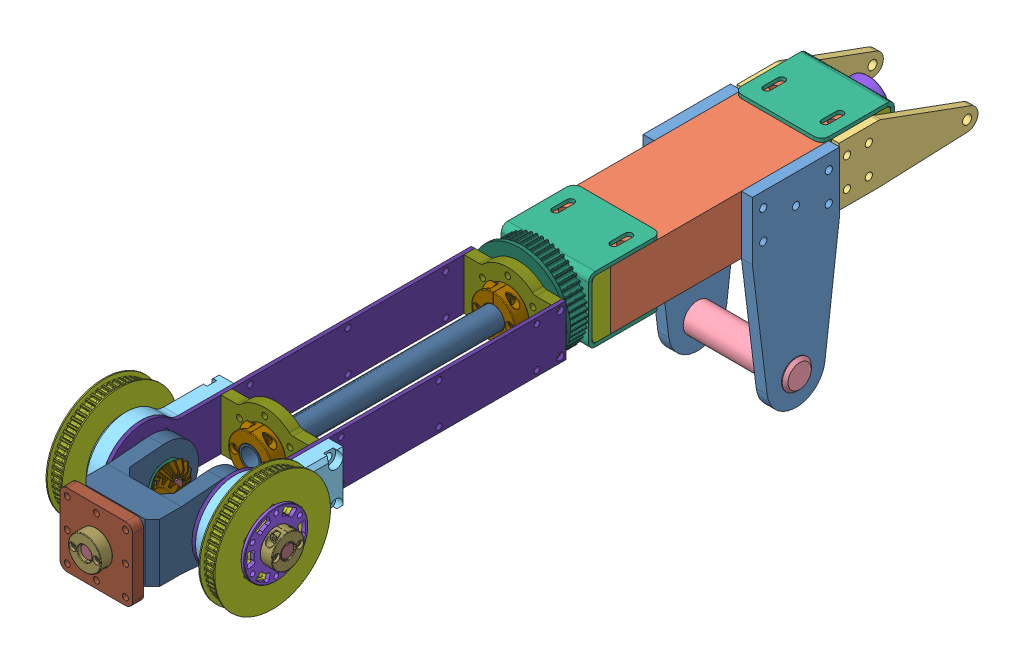
SolidWorks assembly Forearm, configuration Default. Lengths in mm.
Overall size (174.26 202.9 760.46).
74 component instances, 31 part files, 63 mates.
Components (placement in the parent):
- SidePlate^Forearm-1: SidePlate^Forearm [Default] at origin size (9.52 177.8 76.2) (virtual)
- SidePlate^Forearm-2: SidePlate^Forearm [Default] x (-1 0 0) z (0 0 -1) size (9.52 177.8 76.2) (virtual)
- Box^Forearm-1: Box^Forearm [Default] at origin size (76.2 50.8 228.6) (virtual)
- BackSidePlate^Forearm-1: BackSidePlate^Forearm [Default] at origin size (6.35 73.03 146.68) (virtual)
- BackSidePlate^Forearm-2: BackSidePlate^Forearm [Default] at (82.55 0 0) size (6.35 73.03 146.68) (virtual)
- 6061K602_HARDENED PRECISION STEEL SHAFT-1: 6061K602_HARDENED PRECISION STEEL SHAFT [6061K602] at (0 609.075 0) size (101.6 25.4 25.4)
- 6384K367_BALL BEARING-1: 6384K367_BALL BEARING [6384K367] at (0 736.075 166.624) x (1 0 0) z (0 0 -1) size (44.45 44.45 14.3)
- BearingHolder^Forearm-1: BearingHolder^Forearm [Default] at origin size (76.2 57.15 63.5) (virtual)
- BearingSpacer^Forearm-1: BearingSpacer^Forearm [Default] at origin size (76.2 50.8 22.22) (virtual)
- BearingSpacer^Forearm-2: BearingSpacer^Forearm [Default] at (0 0 76.2) x (-1 0 0) z (0 0 -1) size (76.2 50.8 22.22) (virtual)
- BearingHolder^Forearm-2: BearingHolder^Forearm [Default] at (0 0 76.2) x (-1 0 0) z (0 0 -1) size (76.2 57.15 63.5) (virtual)
- 6384K367_BALL BEARING-2: 6384K367_BALL BEARING [6384K367] at (0 736.075 -90.424) x (-1 0 0) z (0 0 1) size (44.45 44.45 14.3)
- 6435K160_ONE-PIECE CLAMP-ON SHAFT COLLAR-1: 6435K160_ONE-PIECE CLAMP-ON SHAFT COLLAR [6435K16] at (0 736.075 -104.7242) x (1 0 0) z (0 0 -1) size (38.1 38.11 12.77)
- 9677T100_CLAMP-ON SHAFT COLLAR WITH MOUNTING HOLES-1: 9677T100_CLAMP-ON SHAFT COLLAR WITH MOUNTING HOLES [9677T1] at (0 736.075 210.2517) x (0 -1 0) z (0 0 -1) size (38.14 38.1 13.27)
- 89955K599_Tube^Forearm-1: 89955K599_Tube^Forearm [Default] at origin size (19.05 19.05 539.7) (virtual)
- ThrustBase^Forearm-1: ThrustBase^Forearm [Default] at origin size (44.45 44.45 8.27) (virtual)
- 5909K460_THRUST NEEDLE-ROLLER BEARING-1: 5909K460_THRUST NEEDLE-ROLLER BEARING [5909K46] at (0 736.075 182.0545) x (0 0 -1) z (1 0 0) size (0.81 31.75 31.75)
- 5909K330_THRUST NEEDLE-ROLLER BEARING-1: 5909K330_THRUST NEEDLE-ROLLER BEARING [5909K33] at (0 736.075 183.0467) x (1 0 0) z (0 1 0) size (31.75 1.98 31.75)
- 5909K460_THRUST NEEDLE-ROLLER BEARING-2: 5909K460_THRUST NEEDLE-ROLLER BEARING [5909K46] at (0 736.075 184.8517) x (0 0 -1) z (1 0 0) size (0.81 31.75 31.75)
- PulleySupportPlate^Forearm-1: PulleySupportPlate^Forearm [Default] at origin size (63.5 63.5 3.18) (virtual)
- J4Pulley-1: J4Pulley [Default] at (0 736.075 191.2017) x (-1 0 0) z (0 -1 0) size (84.06 20.68 84.06)
- WristHub^Forearm-1: WristHub^Forearm [Default] at origin size (76.2 63.5 9.53) (virtual)
- WristSidePlate^Forearm-1: WristSidePlate^Forearm [Default] at origin size (3.17 69.85 323.15) (virtual)
- WristSidePlate^Forearm-2: WristSidePlate^Forearm [Default] at (79.375 0 0) size (3.17 69.85 323.15) (virtual)
- WristHub^Forearm-2: WristHub^Forearm [Default] at (0 0 212.0233) size (76.2 63.5 9.53) (virtual)
- 9677T100_CLAMP-ON SHAFT COLLAR WITH MOUNTING HOLES-2: 9677T100_CLAMP-ON SHAFT COLLAR WITH MOUNTING HOLES [9677T1] at (0 736.075 422.275) x (0 -1 0) z (0 0 -1) size (38.14 38.1 13.27)
- 6843K130_MTL MITER GEAR--20 DEG PRESSURE ANGLE-1: 6843K130_MTL MITER GEAR--20 DEG PRESSURE ANGLE [6843K13] at (-31.1638 691.933 470.788) x (0 -0.999847 0.017483) z (0 0.017483 0.999847) size (34.68 21.82 34.5)
- 6843K130_MTL MITER GEAR--20 DEG PRESSURE ANGLE-3: 6843K130_MTL MITER GEAR--20 DEG PRESSURE ANGLE [6843K13] at (-11.812 691.933 513.7638) x (0.017483 -0.999847 0) z (0.999847 0.017483 0) size (34.68 21.82 34.5)
- 6384K361_BALL BEARING-1-1: 6384K361_BALL BEARING-1 [6384K361] at (-41.3385 736.075 482.6) x (0 0 1) z (-1 0 0) size (31.75 31.75 11.13)
- 5909K440_THRUST NEEDLE-ROLLER BEARING-1: 5909K440_THRUST NEEDLE-ROLLER BEARING [5909K44] at (-34.5472 736.075 482.6) size (0.81 23.81 23.81)
- 5909K310_THRUST NEEDLE-ROLLER BEARING-1: 5909K310_THRUST NEEDLE-ROLLER BEARING [5909K31] at (-32.7422 736.075 482.6) x (0 1 0) z (0 0 1) size (23.81 1.98 23.81)
- MiterSpacer^Forearm-1: MiterSpacer^Forearm [Default] at origin size (2.03 31.75 31.75) (virtual)
- SidePrintedSupport^Forearm-1: SidePrintedSupport^Forearm [Default] at origin size (15.88 69.85 115.89) (virtual)
- 6384K361_BALL BEARING-1-2: 6384K361_BALL BEARING-1 [6384K361] at (-53.9115 736.075 482.6) x (0 0 1) z (1 0 0) size (31.75 31.75 11.13)
- SidePrintedSupport^Forearm-2: SidePrintedSupport^Forearm [Default] at (0 1472.15 0) x (-1 0 0) z (0 0 1) size (15.88 69.85 115.89) (virtual)
- 6384K361_BALL BEARING-1-3: 6384K361_BALL BEARING-1 [6384K361] at (53.9115 736.075 482.6) x (0 0 -1) z (-1 0 0) size (31.75 31.75 11.13)
- 6384K361_BALL BEARING-1-4: 6384K361_BALL BEARING-1 [6384K361] at (41.3385 736.075 482.6) x (0 0 -1) z (1 0 0) size (31.75 31.75 11.13)
- MiterSpacer^Forearm-2: MiterSpacer^Forearm [Default] at (0 0 965.2) x (-1 0 0) z (0 0 -1) size (2.03 31.75 31.75) (virtual)
- 5909K440_THRUST NEEDLE-ROLLER BEARING-2: 5909K440_THRUST NEEDLE-ROLLER BEARING [5909K44] at (34.5472 736.075 482.6) x (-1 0 0) z (0 0 -1) size (0.81 23.81 23.81)
- 5909K310_THRUST NEEDLE-ROLLER BEARING-2: 5909K310_THRUST NEEDLE-ROLLER BEARING [5909K31] at (32.7422 736.075 482.6) x (0 1 0) z (0 0 1) size (23.81 1.98 23.81)
- 6843K130_MTL MITER GEAR--20 DEG PRESSURE ANGLE-4: 6843K130_MTL MITER GEAR--20 DEG PRESSURE ANGLE [6843K13] at (31.1638 779.7771 469.252) x (0 0.999847 -0.017483) z (0 0.017483 0.999847) size (34.68 21.82 34.5)
- 6391K281_OIL-EMBEDDED SLEEVE BEARING-1: 6391K281_OIL-EMBEDDED SLEEVE BEARING [6391K281] at (-25.8945 736.075 482.6) x (0 0 1) z (-1 0 0) size (31.78 31.78 12.7)
- 6391K281_OIL-EMBEDDED SLEEVE BEARING-2: 6391K281_OIL-EMBEDDED SLEEVE BEARING [6391K281] at (25.8945 736.075 482.6) x (0 0 1) z (-1 0 0) size (31.78 31.78 12.7)
- PulleyHubbed-1: PulleyHubbed [Default] at (-79.0217 736.075 482.6) x (0 0 1) z (-1 0 0) size (101 101 17.18)
  - 60t_x_18mm_Wide_VersaPulley_Kit_HTD_5mm_VersaKeys_217-3200 v2-1: 60t_x_18mm_Wide_VersaPulley_Kit_HTD_5mm_VersaKeys_217-3200 v2 [Default] at origin size (101 101 14)
    - 60t_x_18mm_Wide_VersaPulley_Kit_HTD_5mm_VersaKeys_217-3200 v2.step-1: 60t_x_18mm_Wide_VersaPulley_Kit_HTD_5mm_VersaKeys_217-3200 v2.step [Default] at origin size (101 101 14)
      - 217-3200-001 Rev3.step-1: 217-3200-001 Rev3.step [Default] at (0 0 -7) size (101 101 10.18)
      - 217-3200-001 Rev3.step-2: 217-3200-001 Rev3.step [Default] at (0 0 -17.825) x (-1 0 0) z (0 0 -1) size (101 101 10.18)
  - 1_2_ID_1_8_Keyway_Aluminum_VersaHub_217-2590 v1-1: 1_2_ID_1_8_Keyway_Aluminum_VersaHub_217-2590 v1 [Default] at (0 0 -14.9375) x (0 0 1) z (1 0 0) size (12.7 55.88 55.88)
- SidePulleySpacer^Forearm-1: SidePulleySpacer^Forearm [Default] at origin size (3.81 17.78 17.78) (virtual)
- PulleyHubbed-2: PulleyHubbed [Default] at (79.0217 736.075 482.6) x (0 0 -1) z (1 0 0) size (101 101 17.18)
  - 60t_x_18mm_Wide_VersaPulley_Kit_HTD_5mm_VersaKeys_217-3200 v2-1: 60t_x_18mm_Wide_VersaPulley_Kit_HTD_5mm_VersaKeys_217-3200 v2 [Default] at origin size (101 101 14)
    - 60t_x_18mm_Wide_VersaPulley_Kit_HTD_5mm_VersaKeys_217-3200 v2.step-1: 60t_x_18mm_Wide_VersaPulley_Kit_HTD_5mm_VersaKeys_217-3200 v2.step [Default] at origin size (101 101 14)
      - 217-3200-001 Rev3.step-1: 217-3200-001 Rev3.step [Default] at (0 0 -7) size (101 101 10.18)
      - 217-3200-001 Rev3.step-2: 217-3200-001 Rev3.step [Default] at (0 0 -17.825) x (-1 0 0) z (0 0 -1) size (101 101 10.18)
  - 1_2_ID_1_8_Keyway_Aluminum_VersaHub_217-2590 v1-1: 1_2_ID_1_8_Keyway_Aluminum_VersaHub_217-2590 v1 [Default] at (0 0 -14.9375) x (0 0 1) z (1 0 0) size (12.7 55.88 55.88)
- SidePulleySpacer^Forearm-2: SidePulleySpacer^Forearm [Default] at (0 0 965.2) x (-1 0 0) z (0 0 -1) size (3.81 17.78 17.78) (virtual)
- WristBase^Forearm-3: WristBase^Forearm [Default] at origin size (64.49 57.15 92.08) (virtual)
- 6384K361_BALL BEARING-1-5: 6384K361_BALL BEARING-1 [6384K361] at (0 736.075 523.9385) size (31.75 31.75 11.13)
- MiterSpacer^Forearm-3: MiterSpacer^Forearm [Default] at (-482.6 0 482.6) x (0 0 -1) z (1 0 0) size (2.03 31.75 31.75) (virtual)
- 5909K440_THRUST NEEDLE-ROLLER BEARING-3: 5909K440_THRUST NEEDLE-ROLLER BEARING [5909K44] at (0 736.075 517.1472) x (0 0 -1) z (1 0 0) size (0.81 23.81 23.81)
- 5909K310_THRUST NEEDLE-ROLLER BEARING-3: 5909K310_THRUST NEEDLE-ROLLER BEARING [5909K31] at (0 736.075 515.3422) x (0 1 0) z (-1 0 0) size (23.81 1.98 23.81)
- 6384K361_BALL BEARING-1-6: 6384K361_BALL BEARING-1 [6384K361] at (0 736.075 542.8615) x (1 0 0) z (0 0 -1) size (31.75 31.75 11.13)
- MiterSpacer^Forearm-4: MiterSpacer^Forearm [Default] at (-482.6 0 513.0768) x (0 0 -1) z (1 0 0) size (2.03 31.75 31.75) (virtual)
- 5909K440_THRUST NEEDLE-ROLLER BEARING-4: 5909K440_THRUST NEEDLE-ROLLER BEARING [5909K44] at (0 736.075 550.4656) x (0 0 -1) z (1 0 0) size (0.81 23.81 23.81)
- 5909K440_THRUST NEEDLE-ROLLER BEARING-5: 5909K440_THRUST NEEDLE-ROLLER BEARING [5909K44] at (0 736.075 553.2628) x (0 0 -1) z (1 0 0) size (0.81 23.81 23.81)
- 5909K310_THRUST NEEDLE-ROLLER BEARING-4: 5909K310_THRUST NEEDLE-ROLLER BEARING [5909K31] at (0 736.075 551.4578) x (0 1 0) z (-1 0 0) size (23.81 1.98 23.81)
- HandPlate^Forearm-1: HandPlate^Forearm [Default] at origin size (63.5 63.5 9.52) (virtual)
- 9677T210_CLAMP-ON SHAFT COLLAR WITH MOUNTING HOLES-1: 9677T210_CLAMP-ON SHAFT COLLAR WITH MOUNTING HOLES [9677T21] at (0 736.075 567.9472) x (0 1 0) z (0 0 -1) size (28.6 28.57 10.69)
- 9677T210_CLAMP-ON SHAFT COLLAR WITH MOUNTING HOLES-2: 9677T210_CLAMP-ON SHAFT COLLAR WITH MOUNTING HOLES [9677T21] at (-81.9436 736.075 482.6) x (0 -1 0) z (1 0 0) size (28.6 28.57 10.69)
- 9677T210_CLAMP-ON SHAFT COLLAR WITH MOUNTING HOLES-3: 9677T210_CLAMP-ON SHAFT COLLAR WITH MOUNTING HOLES [9677T21] at (81.9436 736.075 482.6) x (0 -1 0) z (-1 0 0) size (28.6 28.57 10.69)
- 8488T310_FULLY KEYED PRECISION DRIVE SHAFT W CERT-1: 8488T310_FULLY KEYED PRECISION DRIVE SHAFT W CERT [8488T31] at (-48.5172 736.075 482.6) x (0 0 1) z (-1 0 0) size (12.7 12.5 76.2)
- 8488T310_FULLY KEYED PRECISION DRIVE SHAFT W CERT-2: 8488T310_FULLY KEYED PRECISION DRIVE SHAFT W CERT [8488T31] at (48.5172 736.075 482.6) x (0 0 1) z (-1 0 0) size (12.7 12.5 76.2)
- 8488T310_FULLY KEYED PRECISION DRIVE SHAFT W CERT-3: 8488T310_FULLY KEYED PRECISION DRIVE SHAFT W CERT [8488T31] at (0 736.075 532.819) size (12.7 12.5 76.2)
Mates (geometry in assembly coordinates):
- Concentric1: concentric anti-aligned: cylinder of SidePlate^Forearm-1 through (-47.625 609.075 0) axis (1 0 0) radius 12.7; circle of 6061K602_HARDENED PRECISION STEEL SHAFT-1
- Width1: width anti-aligned: plane of 6061K602_HARDENED PRECISION STEEL SHAFT-1 through (-50.8 609.075 0) normal (-1 0 0); plane of SidePlate^Forearm-2 through (50.8 609.075 0) normal (1 0 0); plane of 6061K602_HARDENED PRECISION STEEL SHAFT-1 through (47.625 609.075 0) normal (1 0 0); plane of SidePlate^Forearm-1 through (-47.625 609.075 0) normal (-1 0 0)
- Concentric2: concentric aligned: cylinder of 6384K367_BALL BEARING-1 through (0 736.075 160.274) axis (0 0 -1) radius 20.6375; cylinder of BearingHolder^Forearm-1 through (0 736.075 171.45) axis (0 0 -1) radius 20.6375
- Coincident2: coincident anti-aligned: plane of 6384K367_BALL BEARING-1 through (0 720.6646 171.45) normal (0 0 -1); plane of BearingHolder^Forearm-1 through (0 0 171.45) normal (0 0 1)
- Concentric3: concentric aligned: cylinder of 6384K367_BALL BEARING-2 through (0 736.075 -84.074) axis (0 0 1) radius 9.525; cylinder of 6435K160_ONE-PIECE CLAMP-ON SHAFT COLLAR-1 through (0 736.075 -111.0742) axis (0 0 1) radius 9.525
- Coincident3: coincident anti-aligned: plane of 6384K367_BALL BEARING-2 through (0 725.2038 -98.3742) normal (0 0 -1); plane of 6435K160_ONE-PIECE CLAMP-ON SHAFT COLLAR-1 through (0 736.075 -98.3742) normal (0 0 1)
- Concentric4: concentric anti-aligned: cylinder of 6384K367_BALL BEARING-1 through (0 736.075 160.274) axis (0 0 -1) radius 9.525; cylinder of 9677T100_CLAMP-ON SHAFT COLLAR WITH MOUNTING HOLES-1 through (0 736.075 203.9017) axis (0 0 1) radius 9.525
- Concentric5: concentric anti-aligned: cylinder of 89955K599_Tube^Forearm-1 through (0 736.075 455.5658) axis (0 0 -1) radius 9.525; cylinder of 5909K460_THRUST NEEDLE-ROLLER BEARING-1 through (0 736.075 181.2417) axis (0 0 1) radius 9.5504
- Coincident4: coincident anti-aligned: plane of ThrustBase^Forearm-1 through (0 736.075 181.2417) normal (0 0 1); plane of 5909K460_THRUST NEEDLE-ROLLER BEARING-1 through (0 736.075 181.2417) normal (0 0 -1)
- Concentric6: concentric anti-aligned: cylinder of 89955K599_Tube^Forearm-1 through (0 736.075 455.5658) axis (0 0 -1) radius 9.525; cylinder of 5909K330_THRUST NEEDLE-ROLLER BEARING-1 through (0 736.075 184.0389) axis (0 0 1) radius 9.5504
- Tangent1: tangent anti-aligned: plane of 5909K460_THRUST NEEDLE-ROLLER BEARING-1 through (0 736.075 182.0545) normal (0 0 1); cylinder of 5909K330_THRUST NEEDLE-ROLLER BEARING-1 through (-5.4469 722.3178 183.0467) axis (-0.368125 -0.929776 0) radius 0.9922
- Concentric7: concentric anti-aligned: cylinder of 89955K599_Tube^Forearm-1 through (0 736.075 455.5658) axis (0 0 -1) radius 9.525; cylinder of 5909K460_THRUST NEEDLE-ROLLER BEARING-2 through (0 736.075 184.0389) axis (0 0 1) radius 9.5504
- Tangent2: tangent anti-aligned: cylinder of 5909K330_THRUST NEEDLE-ROLLER BEARING-1 through (-1.8545 721.3954 183.0467) axis (-0.125333 -0.992115 0) radius 0.9922; plane of 5909K460_THRUST NEEDLE-ROLLER BEARING-2 through (0 736.075 184.0389) normal (0 0 -1)
- Concentric8: concentric anti-aligned: cylinder of 89955K599_Tube^Forearm-1 through (0 736.075 455.5658) axis (0 0 -1) radius 9.525; circle of J4Pulley-1
- Coincident6: coincident anti-aligned: plane of PulleySupportPlate^Forearm-1 through (0 0 188.0267) normal (0 0 1); plane of J4Pulley-1 through (0 736.075 188.0267) normal (0 0 -1)
- Parallel1: parallel anti-aligned: plane of 9677T100_CLAMP-ON SHAFT COLLAR WITH MOUNTING HOLES-1 through (0.0953 755.1248 203.9017) normal (-1 0 0)
- Coincident11: coincident anti-aligned: plane of 9677T100_CLAMP-ON SHAFT COLLAR WITH MOUNTING HOLES-1 through (0 736.075 203.9017) normal (0 0 -1); plane of WristBase^Forearm-1 through (-24.5934 763.0625 203.9017) normal (0 0 1)
- Concentric10: concentric aligned: cylinder of 89955K599_Tube^Forearm-1 through (0 736.075 455.5658) axis (0 0 -1) radius 9.525; cylinder of WristHub^Forearm-2 through (0 736.075 415.925) axis (0 0 -1) radius 9.525
- Distance2: distance = 406.4 mm: plane of assembly through (0 0 0) normal (0 0 1); plane of WristBase^Forearm-2 through (-24.5934 763.0625 406.4) normal (0 0 -1)
- Concentric11: concentric anti-aligned: cylinder of 89955K599_Tube^Forearm-1 through (0 736.075 455.5658) axis (0 0 -1) radius 7.9375; cylinder of 9677T100_CLAMP-ON SHAFT COLLAR WITH MOUNTING HOLES-2 through (0 736.075 415.925) axis (0 0 1) radius 9.525
- Coincident13: coincident anti-aligned: plane of WristHub^Forearm-2 through (-24.5934 763.0625 415.925) normal (0 0 1); plane of 9677T100_CLAMP-ON SHAFT COLLAR WITH MOUNTING HOLES-2 through (0 736.075 415.925) normal (0 0 -1)
- Concentric12: concentric anti-aligned: cylinder of WristSidePlate^Forearm-1 through (-41.275 736.075 482.6) axis (1 0 0) radius 14.2875; cylinder of 6843K130_MTL MITER GEAR--20 DEG PRESSURE ANGLE-1 through (31.0355 736.075 482.6) axis (-1 0 0) radius 6.3563
- Concentric13: concentric anti-aligned: cylinder of 89955K599_Tube^Forearm-1 through (0 736.075 455.5658) axis (0 0 -1) radius 7.9375; cylinder of 6843K130_MTL MITER GEAR--20 DEG PRESSURE ANGLE-3 through (0 736.075 451.5645) axis (0 0 1) radius 6.3563
- Distance3: distance = 31.75 mm: cylinder of 6843K130_MTL MITER GEAR--20 DEG PRESSURE ANGLE-3 through (0 736.075 451.5645) axis (0 0 1) radius 6.3563; plane of 6843K130_MTL MITER GEAR--20 DEG PRESSURE ANGLE-1 through (-31.75 735.853 469.9019) normal (-1 0 0)
- Distance4: distance = 31.75 mm: plane of 6843K130_MTL MITER GEAR--20 DEG PRESSURE ANGLE-3 through (-12.6981 735.853 514.35) normal (0 0 1); cylinder of 6843K130_MTL MITER GEAR--20 DEG PRESSURE ANGLE-1 through (31.0355 736.075 482.6) axis (-1 0 0) radius 6.3563
- Concentric14: concentric anti-aligned: cylinder of WristSidePlate^Forearm-1 through (-41.275 736.075 482.6) axis (1 0 0) radius 14.2875; cylinder of 6384K361_BALL BEARING-1-1 through (-46.101 736.075 482.6) axis (-1 0 0) radius 14.2875
- Coincident14: coincident anti-aligned: plane of WristSidePlate^Forearm-1 through (-38.1 701.15 450.2212) normal (1 0 0); plane of 6384K361_BALL BEARING-1-1 through (-38.1 746.7938 482.6) normal (-1 0 0)
- Concentric15: concentric aligned: cylinder of 6843K130_MTL MITER GEAR--20 DEG PRESSURE ANGLE-1 through (31.0355 736.075 482.6) axis (-1 0 0) radius 6.3563; cylinder of 5909K440_THRUST NEEDLE-ROLLER BEARING-1 through (-33.7344 736.075 482.6) axis (-1 0 0) radius 6.3754
- Concentric16: concentric anti-aligned: cylinder of 6843K130_MTL MITER GEAR--20 DEG PRESSURE ANGLE-1 through (31.0355 736.075 482.6) axis (-1 0 0) radius 6.3563; cylinder of 5909K310_THRUST NEEDLE-ROLLER BEARING-1 through (-31.75 736.075 482.6) axis (1 0 0) radius 6.3754
- Tangent6: tangent anti-aligned: plane of 6843K130_MTL MITER GEAR--20 DEG PRESSURE ANGLE-1 through (-31.75 735.853 469.9019) normal (-1 0 0); cylinder of 5909K310_THRUST NEEDLE-ROLLER BEARING-1 through (-32.7422 725.194 485.3554) axis (0 -0.9694 0.245485) radius 0.9922
- Tangent7: tangent anti-aligned: plane of 5909K440_THRUST NEEDLE-ROLLER BEARING-1 through (-33.7344 736.075 482.6) normal (1 0 0); cylinder of 5909K310_THRUST NEEDLE-ROLLER BEARING-1 through (-32.7422 725.194 485.3554) axis (0 -0.9694 0.245485) radius 0.9922
- Concentric17: concentric aligned: cylinder of SidePrintedSupport^Forearm-1 through (-57.15 736.075 482.6) axis (1 0 0) radius 14.2875; cylinder of 6384K361_BALL BEARING-1-2 through (-49.149 736.075 482.6) axis (1 0 0) radius 14.2875
- Coincident16: coincident anti-aligned: plane of SidePrintedSupport^Forearm-1 through (-57.15 0 0) normal (-1 0 0); plane of 6384K361_BALL BEARING-1-2 through (-57.15 725.3562 482.6) normal (1 0 0)
- Concentric18: concentric anti-aligned: cylinder of 6843K130_MTL MITER GEAR--20 DEG PRESSURE ANGLE-1 through (31.0355 736.075 482.6) axis (-1 0 0) radius 12.7; cylinder of 6391K281_OIL-EMBEDDED SLEEVE BEARING-1 through (-32.2445 736.075 482.6) axis (1 0 0) radius 12.7
- Concentric20: concentric anti-aligned: cylinder of 6384K361_BALL BEARING-1-2 through (-49.149 736.075 482.6) axis (1 0 0) radius 6.35; cylinder of PulleyHubbed-1/1_2_ID_1_8_Keyway_Aluminum_VersaHub_217-2590 v1-1 through (-64.0842 736.075 482.6) axis (-1 0 0) radius 6.3627
- Coincident18: coincident anti-aligned: plane of PulleyHubbed-1/1_2_ID_1_8_Keyway_Aluminum_VersaHub_217-2590 v1-1 through (-64.0842 736.075 482.6) normal (1 0 0); plane of SidePulleySpacer^Forearm-1 through (-64.0842 736.075 482.6) normal (-1 0 0)
- Concentric21: concentric anti-aligned: cylinder of WristBase^Forearm-3 through (0 736.075 546.1) axis (0 0 -1) radius 14.2875; cylinder of 6384K361_BALL BEARING-1-5 through (0 736.075 528.701) axis (0 0 1) radius 14.2875
- Coincident19: coincident anti-aligned: plane of WristBase^Forearm-3 through (0 0 520.7) normal (0 0 -1); plane of 6384K361_BALL BEARING-1-5 through (0 746.7938 520.7) normal (0 0 1)
- Concentric22: concentric anti-aligned: cylinder of WristBase^Forearm-3 through (0 736.075 546.1) axis (0 0 -1) radius 14.2875; cylinder of MiterSpacer^Forearm-3 through (0 736.075 472.2459) axis (0 0 1) radius 9.3726
- Coincident21: coincident anti-aligned: plane of 6384K361_BALL BEARING-1-5 through (0 749.8863 519.176) normal (0 0 -1); plane of MiterSpacer^Forearm-3 through (0 736.075 519.176) normal (0 0 1)
- Concentric23: concentric anti-aligned: cylinder of WristBase^Forearm-3 through (0 736.075 546.1) axis (0 0 -1) radius 14.2875; cylinder of 5909K440_THRUST NEEDLE-ROLLER BEARING-3 through (0 736.075 516.3344) axis (0 0 1) radius 6.3754
- Coincident22: coincident anti-aligned: plane of MiterSpacer^Forearm-3 through (0 736.075 517.1472) normal (0 0 -1); plane of 5909K440_THRUST NEEDLE-ROLLER BEARING-3 through (0 736.075 517.1472) normal (0 0 1)
- Concentric24: concentric anti-aligned: cylinder of WristBase^Forearm-3 through (0 736.075 546.1) axis (0 0 -1) radius 14.2875; cylinder of 5909K310_THRUST NEEDLE-ROLLER BEARING-3 through (0 736.075 516.3344) axis (0 0 1) radius 6.3754
- Tangent8: tangent anti-aligned: plane of 6843K130_MTL MITER GEAR--20 DEG PRESSURE ANGLE-3 through (-12.6981 735.853 514.35) normal (0 0 1); cylinder of 5909K310_THRUST NEEDLE-ROLLER BEARING-3 through (-8.8576 742.9692 515.3422) axis (-0.789141 0.614213 0) radius 0.9922
- Concentric25: concentric aligned: cylinder of WristBase^Forearm-3 through (0 736.075 546.1) axis (0 0 -1) radius 14.2875; cylinder of 6384K361_BALL BEARING-1-6 through (0 736.075 538.099) axis (0 0 -1) radius 14.2875
- Coincident24: coincident anti-aligned: plane of WristBase^Forearm-3 through (0 0 546.1) normal (0 0 1); plane of 6384K361_BALL BEARING-1-6 through (0 725.3562 546.1) normal (0 0 -1)
- Concentric26: concentric anti-aligned: cylinder of 6384K361_BALL BEARING-1-6 through (0 736.075 538.099) axis (0 0 -1) radius 6.35; cylinder of MiterSpacer^Forearm-4 through (0 736.075 502.7227) axis (0 0 1) radius 9.3726
- Coincident25: coincident anti-aligned: plane of 6384K361_BALL BEARING-1-6 through (0 722.2637 547.624) normal (0 0 1); plane of MiterSpacer^Forearm-4 through (0 736.075 547.624) normal (0 0 -1)
- Concentric27: concentric anti-aligned: cylinder of 6384K361_BALL BEARING-1-6 through (0 736.075 538.099) axis (0 0 -1) radius 6.35; cylinder of 5909K440_THRUST NEEDLE-ROLLER BEARING-4 through (0 736.075 549.6528) axis (0 0 1) radius 6.3754
- Coincident26: coincident anti-aligned: plane of MiterSpacer^Forearm-4 through (0 736.075 549.6528) normal (0 0 1); plane of 5909K440_THRUST NEEDLE-ROLLER BEARING-4 through (0 736.075 549.6528) normal (0 0 -1)
- Concentric28: concentric anti-aligned: cylinder of 6384K361_BALL BEARING-1-6 through (0 736.075 538.099) axis (0 0 -1) radius 6.35; cylinder of 5909K310_THRUST NEEDLE-ROLLER BEARING-4 through (0 736.075 552.45) axis (0 0 1) radius 6.3754
- Tangent9: tangent anti-aligned: plane of 5909K440_THRUST NEEDLE-ROLLER BEARING-4 through (0 736.075 550.4656) normal (0 0 1); cylinder of 5909K310_THRUST NEEDLE-ROLLER BEARING-4 through (-6.1392 726.6783 551.4578) axis (-0.546948 -0.837166 0) radius 0.9922
- Tangent10: tangent anti-aligned: plane of 5909K440_THRUST NEEDLE-ROLLER BEARING-5 through (0 736.075 552.45) normal (0 0 -1); cylinder of 5909K310_THRUST NEEDLE-ROLLER BEARING-4 through (-2.7554 725.194 551.4578) axis (-0.245485 -0.9694 0) radius 0.9922
- Concentric29: concentric anti-aligned: cylinder of 6384K361_BALL BEARING-1-6 through (0 736.075 538.099) axis (0 0 -1) radius 6.35; cylinder of 5909K440_THRUST NEEDLE-ROLLER BEARING-5 through (0 736.075 552.45) axis (0 0 1) radius 6.3754
- Concentric39: concentric anti-aligned: cylinder of HandPlate^Forearm-1 through (0 736.075 562.7878) axis (0 0 -1) radius 6.35; cylinder of 9677T210_CLAMP-ON SHAFT COLLAR WITH MOUNTING HOLES-1 through (0 736.075 562.7878) axis (0 0 1) radius 6.35
- Coincident29: coincident anti-aligned: plane of HandPlate^Forearm-1 through (0 0 562.7878) normal (0 0 1); plane of 9677T210_CLAMP-ON SHAFT COLLAR WITH MOUNTING HOLES-1 through (0 736.075 562.7878) normal (0 0 -1)
- Concentric40: concentric aligned: cylinder of PulleyHubbed-1/1_2_ID_1_8_Keyway_Aluminum_VersaHub_217-2590 v1-1 through (-64.0842 736.075 482.6) axis (-1 0 0) radius 6.3627; cylinder of 9677T210_CLAMP-ON SHAFT COLLAR WITH MOUNTING HOLES-2 through (-76.7842 736.075 482.6) axis (-1 0 0) radius 6.35
- Coincident30: coincident anti-aligned: plane of PulleyHubbed-1/1_2_ID_1_8_Keyway_Aluminum_VersaHub_217-2590 v1-1 through (-76.7842 704.5282 482.6) normal (-1 0 0); plane of 9677T210_CLAMP-ON SHAFT COLLAR WITH MOUNTING HOLES-2 through (-76.7842 736.075 482.6) normal (1 0 0)
- Concentric41: concentric anti-aligned: cylinder of 6384K361_BALL BEARING-1-1 through (-46.101 736.075 482.6) axis (-1 0 0) radius 6.35; cylinder of 8488T310_FULLY KEYED PRECISION DRIVE SHAFT W CERT-1 through (-86.6172 736.075 482.6) axis (1 0 0) radius 6.35
- Width2: width anti-aligned: plane of 8488T310_FULLY KEYED PRECISION DRIVE SHAFT W CERT-1 through (-86.6172 736.075 482.6) normal (-1 0 0); plane of 8488T310_FULLY KEYED PRECISION DRIVE SHAFT W CERT-1 through (-10.4172 736.075 482.6) normal (1 0 0); plane of 6843K130_MTL MITER GEAR--20 DEG PRESSURE ANGLE-1 through (-9.9314 735.9639 476.2446) normal (1 0 0); plane of 9677T210_CLAMP-ON SHAFT COLLAR WITH MOUNTING HOLES-2 through (-87.1029 736.075 482.6) normal (-1 0 0)
- Coincident32: coincident anti-aligned: circle of 6843K130_MTL MITER GEAR--20 DEG PRESSURE ANGLE-1; plane of 6391K281_OIL-EMBEDDED SLEEVE BEARING-1 through (-19.5445 736.075 482.6) normal (1 0 0)
- Concentric42: concentric anti-aligned: cylinder of 9677T210_CLAMP-ON SHAFT COLLAR WITH MOUNTING HOLES-1 through (0 736.075 562.7878) axis (0 0 1) radius 6.35; cylinder of 8488T310_FULLY KEYED PRECISION DRIVE SHAFT W CERT-3 through (0 736.075 570.919) axis (0 0 -1) radius 6.35
- Width3: width aligned: plane of 8488T310_FULLY KEYED PRECISION DRIVE SHAFT W CERT-3 through (0 736.075 570.919) normal (0 0 1); plane of 9677T210_CLAMP-ON SHAFT COLLAR WITH MOUNTING HOLES-1 through (0 736.075 494.719) normal (0 0 -1); plane of 8488T310_FULLY KEYED PRECISION DRIVE SHAFT W CERT-3 through (0 736.075 573.1065) normal (0 0 1); plane of 6843K130_MTL MITER GEAR--20 DEG PRESSURE ANGLE-3 through (-6.3554 735.9639 492.5314) normal (0 0 -1)
